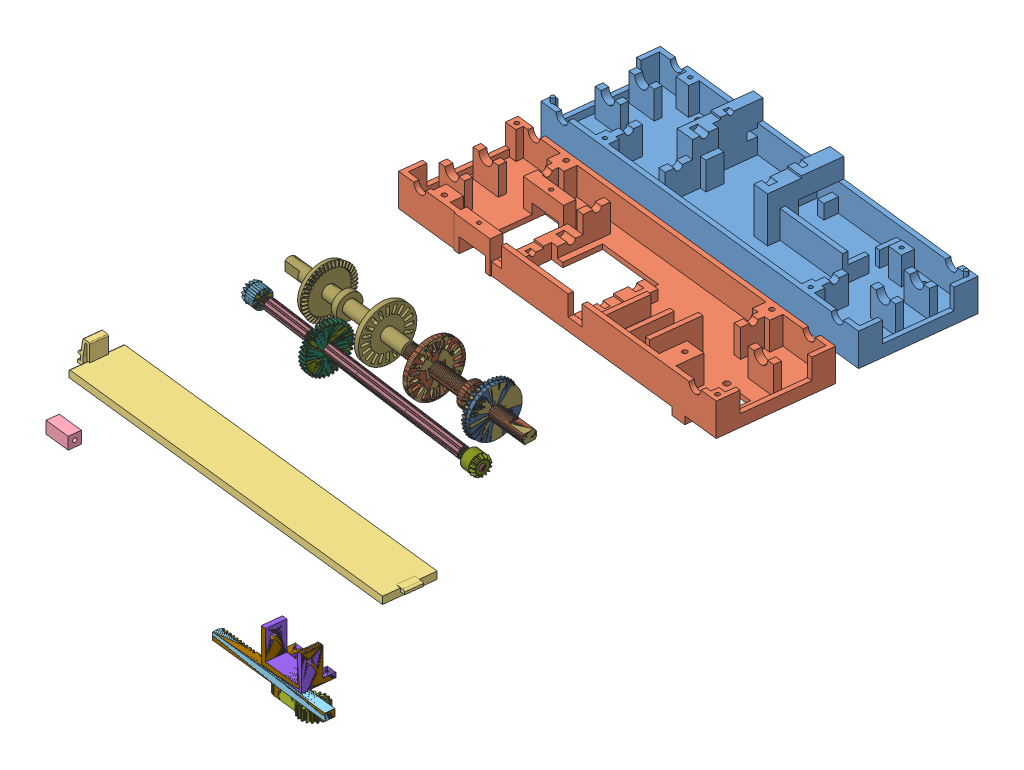
SolidWorks assembly 电机组打印, configuration 默认. Lengths in mm.
Overall size (183.34 34.53 292.08).
24 component instances, 16 part files, 28 mates.
Components (placement in the parent):
- 电机上盖-1: 电机上盖 [默认] at (-7.8094 0 164.4775) x (0.993706 0 0.112024) z (-0.112024 0 0.993706) size (150 21.7 45)
- 电机下盖-1: 电机下盖 [默认] at (-12.2413 2 219.3263) x (0.993706 0 0.112024) z (0.112024 0 -0.993706) size (150 19.2 45.45)
- 电池底板-1: 电池底板 [默认] at (-31.1405 -8.9006 352.0222) x (0.993706 0 0.112024) z (-0.112024 0 0.993706) size (154.64 10.19 20.6)
- 电路板支柱-1: 电路板支柱 [默认] at (-70.6784 2.5 386.7313) x (0.112024 0 -0.993706) z (0 1 0) size (5 10.5 5)
- 变速杆齿轮零件-1: 变速杆齿轮零件 [默认] at (51.4079 48.923 421.3552) x (0.993705 -0.000261 0.112024) z (-0.112024 0 0.993706) size (53 3 3.8) (hidden)
- 矩形连接件-1: 矩形连接件 [默认] at (56.5986 -4.8283 421.1405) x (-0.112024 0 0.993706) z (0.000259 1 0.000029) size (2 1 1) (hidden)
- 矩形连接件-2: 矩形连接件 [默认] at (53.9998 -8.8277 422.7596) x (0.112024 0 -0.993706) z (0.000259 1 0.000029) size (2 1 1) (hidden)
- 舵机齿轮连动件-1: 舵机齿轮连动件 [默认] at (62.0528 -12.8297 420.0519) x (0.997269 -0.000261 0.073848) z (0.000259 1 0.000029) size (22.76 10.91 4) (hidden)
- 变速杆-1: 变速杆 [默认] at (53.0022 -3.8272 415.5525) x (-0.112024 0 0.993706) z (0.000259 1 0.000029) size (12.9 19 14) (hidden)
- 小零件打印体-1: 小零件打印体 [默认] at (-256.8464 53.2641 -116.465) size (53.09 23.01 16.18)
- 矩形连接件-3: 矩形连接件 [默认] at (-36.5871 -0.6015 283.7988) x (0.021774 0.980928 -0.193147) z (0.993706 0 0.112024) size (2 1 1) (hidden)
- 车轴带锥齿后轴-3: 车轴带锥齿后轴 [默认] at (7.2186 -8.2651 241.138) x (-0.007497 0.997119 0.075482) z (-0.317112 -0.073959 0.9455) (hidden)
  - 42锥齿轮X5-1: 42锥齿轮X5 [GB - Straight bevel gear 0.5M 42GT 14PT 20PA 2FW ---42O20H6MD5.0N] at (11.6891 -10.019 43.5574) x (-0.001006 0.977873 0.209198) z (-0.649532 0.158421 -0.743647) size (3.43 21.19 21.21) (hidden)
  - 车轮连杆带齿轮后轴-1: 车轮连杆带齿轮后轴 [默认] at (11.6997 -20.3376 41.3499) x (0.999995 0.000336 0.003235) z (-0.003093 -0.2092 0.977868) size (22 56 22) (hidden)
- 车轴带锥齿后轴-1: 车轴带锥齿后轴 [默认] at (-75.2178 44.6532 289.4813) x (0.111024 0.003093 -0.993813) z (0.208243 -0.977868 0.02022) (hidden)
  - 42锥齿轮X5-1: 42锥齿轮X5 [GB - Straight bevel gear 0.5M 42GT 14PT 20PA 2FW ---42O20H6MD5.0N] at (11.6891 -10.019 43.5574) x (-0.001006 0.977873 0.209198) z (-0.649532 0.158421 -0.743647) size (3.43 21.19 21.21) (hidden)
  - 车轮连杆带齿轮后轴-1: 车轮连杆带齿轮后轴 [默认] at (11.6997 -20.3376 41.3499) x (0.999995 0.000336 0.003235) z (-0.003093 -0.2092 0.977868) size (22 56 22) (hidden)
- 车轮打印-1: 车轮打印 [默认] at (65.5103 -39.1592 81.5476) size (112.82 22 29.53)
- 横向传动轴带锥齿-1: 横向传动轴带锥齿 [默认] at (-5.661 26.6876 198.0927) x (-0.013001 0.987555 0.156734) z (-0.131578 -0.157074 0.978782) size (20.6 113.01 20.6) (hidden)
  - 横向传动轴-1: 横向传动轴 [默认] at (-4.8278 9.9238 112) size (4.5 112.35 4.5)
  - 前后传动锥齿14-1: 前后传动锥齿14 [GB - Straight bevel pinion 0.5M14PT 42GT 20PA 2FW ---14O7.5H14MD3.0N] at (-4.8278 64.1735 112) x (0 1 0) z (-0.872078 0 0.489366) size (6.25 8.01 8.21) (hidden)
  - 前后传动锥齿14-2: 前后传动锥齿14 [GB - Straight bevel pinion 0.5M14PT 42GT 20PA 2FW ---14O7.5H14MD3.0N] at (-4.8278 -44.326 112) x (0 -1 0) z (0.420943 0 -0.907087) size (6.25 8.01 8.21)
  - 横向传动齿轮36x3-1: 横向传动齿轮36x3 [默认] at (-4.8278 28.1488 112) x (0.995885 0 0.090621) z (0 1 0) size (18.96 18.96 5.5)
- 横向传动轴带齿轮零件-1: 横向传动轴带齿轮零件 [默认] x (1 0 0) z (0 1 0) size (112.89 23.38 19.02)
Mates (geometry in assembly coordinates):
- 重合1: coincident anti-aligned: plane of 电机上盖-1 through (-7.8094 0 164.4775) normal (0 -1 0)
- 重合2: coincident aligned: plane of 电机上盖-1 through (-7.8094 0 164.4775) normal (0 -1 0); plane of 电机下盖-1 through (-12.2413 0 219.3263) normal (0 -1 0)
- 距离1: distance = 10 mm anti-aligned: plane of 电机下盖-1 through (-84.2487 0 188.5661) normal (0.112024 0 -0.993706); plane of 电机上盖-1 through (-84.8579 2 178.4341) normal (-0.112024 0 0.993706)
- 重合23: coincident aligned: plane of 电机下盖-1 through (-12.2413 0 219.3263) normal (0 -1 0); plane of 电路板支柱-1 through (-81.3923 0 388.0393) normal (0 -1 0)
- 平行2: parallel aligned: plane of 电机下盖-1 through (-89.2897 0 233.2828) normal (-0.112024 0 0.993706); plane of 变速杆齿轮零件-1 through (35.7088 -7.8229 421.6536) normal (-0.112024 0 0.993706)
- 平行3: parallel aligned: plane of 电机下盖-1 through (-89.2897 0 233.2828) normal (-0.112024 0 0.993706); plane of 电路板支柱-1 through (-81.3923 0 388.0393) normal (-0.112024 0 0.993706)
- 宽度1: width aligned: plane of 矩形连接件-1 through (55.6848 -3.8281 422.9999) normal (-0.112024 0 0.993706); plane of 变速杆齿轮零件-1 through (55.9088 -3.8281 421.0125) normal (0.112024 0 -0.993706); plane of 矩形连接件-1 through (35.7088 -7.8229 421.6536) normal (-0.112024 0 0.993706); plane of 变速杆齿轮零件-1 through (36.1345 -7.8229 417.8775) normal (0.112024 0 -0.993706)
- 重合28: coincident anti-aligned: plane of 变速杆齿轮零件-1 through (72.6895 -4.8326 423.9105) normal (0.000259 1 0.000029); plane of 矩形连接件-1 through (56.5986 -4.8283 421.1405) normal (-0.000259 -1 -0.000029)
- 距离2: distance = 17 mm aligned: plane of 矩形连接件-1 through (55.9088 -3.8281 421.0125) normal (0.993705 -0.000261 0.112024); plane of 变速杆齿轮零件-1 through (72.4759 -7.8326 425.7985) normal (0.993705 -0.000261 0.112024)
- 重合29: coincident aligned: plane of 变速杆-1 through (61.5467 -1.8297 424.5664) normal (-0.112024 0 0.993706); plane of 变速杆齿轮零件-1 through (35.7088 -7.8229 421.6536) normal (-0.112024 0 0.993706)
- 重合30: coincident anti-aligned: plane of 变速杆-1 through (53.0022 -3.8272 415.5525) normal (-0.000259 -1 -0.000029); plane of 矩形连接件-1 through (56.5988 -3.8283 421.1406) normal (0.000259 1 0.000029)
- 距离3: distance = 6 mm aligned: plane of 矩形连接件-1 through (55.9088 -3.8281 421.0125) normal (0.993705 -0.000261 0.112024); plane of 变速杆-1 through (62.9918 -1.8297 411.7476) normal (0.993705 -0.000261 0.112024)
- 重合32: coincident aligned: plane of 矩形连接件-1 through (55.6848 -3.8281 422.9999) normal (-0.112024 0 0.993706); plane of 矩形连接件-2 through (54.69 -7.8279 422.8877) normal (-0.112024 0 0.993706)
- 重合33: coincident anti-aligned: plane of 变速杆齿轮零件-1 through (72.6888 -7.8326 423.9104) normal (-0.000259 -1 -0.000029); plane of 矩形连接件-2 through (54 -7.8277 422.7596) normal (0.000259 1 0.000029)
- 重合34: coincident aligned: plane of 矩形连接件-1 through (54.9151 -3.8279 420.9004) normal (-0.993705 0.000261 -0.112024); plane of 矩形连接件-2 through (54.69 -7.8279 422.8877) normal (-0.993705 0.000261 -0.112024)
- 重合35: coincident anti-aligned: plane of 舵机齿轮连动件-1 through (62.0538 -8.8297 420.052) normal (0.000259 1 0.000029); plane of 矩形连接件-2 through (53.9998 -8.8277 422.7596) normal (-0.000259 -1 -0.000029)
- 重合36: coincident aligned: plane of 舵机齿轮连动件-1 through (47.5448 -11.326 422.0822) normal (-0.112024 0 0.993706); plane of 矩形连接件-2 through (54.69 -7.8279 422.8877) normal (-0.112024 0 0.993706)
- 距离4: distance = 6 mm: plane of 矩形连接件-2 through (55.6837 -7.8281 422.9997) normal (0.993705 -0.000261 0.112024); cylinder of 舵机齿轮连动件-1 through (62.0538 -8.8297 420.052) axis (-0.000259 -1 -0.000029) radius 5.5
- 重合41: coincident anti-aligned: plane of 矩形连接件-3 through (-36.5871 -0.6015 283.7988) normal (-0.993706 0 -0.112024); plane of 车轴带锥齿后轴-1/车轮连杆带齿轮后轴-1 through (-36.3796 0 281.9582) normal (0.993706 0 0.112024)
- 重合42: coincident aligned: plane of 电机下盖-1 through (-12.2413 0 219.3263) normal (0 -1 0); plane of 车轴带锥齿后轴-1/车轮连杆带齿轮后轴-1 through (-85.0712 0 276.4691) normal (0 -1 0)
- 平行5: parallel anti-aligned: plane of 电机下盖-1 through (-89.2897 0 233.2828) normal (-0.112024 0 0.993706); plane of 车轴带锥齿后轴-1/车轮连杆带齿轮后轴-1 through (-85.0712 0 276.4691) normal (0.112024 0 -0.993706)
- 平行6: parallel anti-aligned: plane of 电机下盖-1 through (-89.2897 0 233.2828) normal (-0.112024 0 0.993706); plane of 电池底板-1 through (-103.5209 -5.9006 333.4972) normal (0.112024 0 -0.993706)
- 同心1: concentric anti-aligned: cylinder of 车轴带锥齿后轴-1/车轮连杆带齿轮后轴-1 through (-36.3796 0 281.9582) axis (-0.993706 0 -0.112024) radius 2.75; cylinder of 车轴带锥齿后轴-3/车轮连杆带齿轮后轴-1 through (-35.3859 0 282.0703) axis (0.993706 0 0.112024) radius 2.75
- 重合43: coincident anti-aligned: plane of 矩形连接件-3 through (-35.5934 -0.6015 283.9108) normal (0.993706 0 0.112024); plane of 车轴带锥齿后轴-3/车轮连杆带齿轮后轴-1 through (-35.3859 0 282.0703) normal (-0.993706 0 -0.112024)
- 在位1: in place: plane of 横向传动轴带齿轮零件-1 through (0 0 0) normal (0 1 0); moOrthogonalPlaneRef_w of 横向传动轴带齿轮零件-1 through (0 0 0) normal (0 0 -1); plane of 横向传动轴带齿轮零件-1 through (0 0 0) normal (1 0 0); unknown of 横向传动轴带齿轮零件-1
- 重合44: coincident aligned: 
- 重合45: coincident aligned: plane of 横向传动轴带齿轮零件-1 through (0 0 0) normal (0 0 -1)
- 重合46: coincident anti-aligned: plane of 横向传动轴带齿轮零件-1 through (0 0 0) normal (1 0 0)
